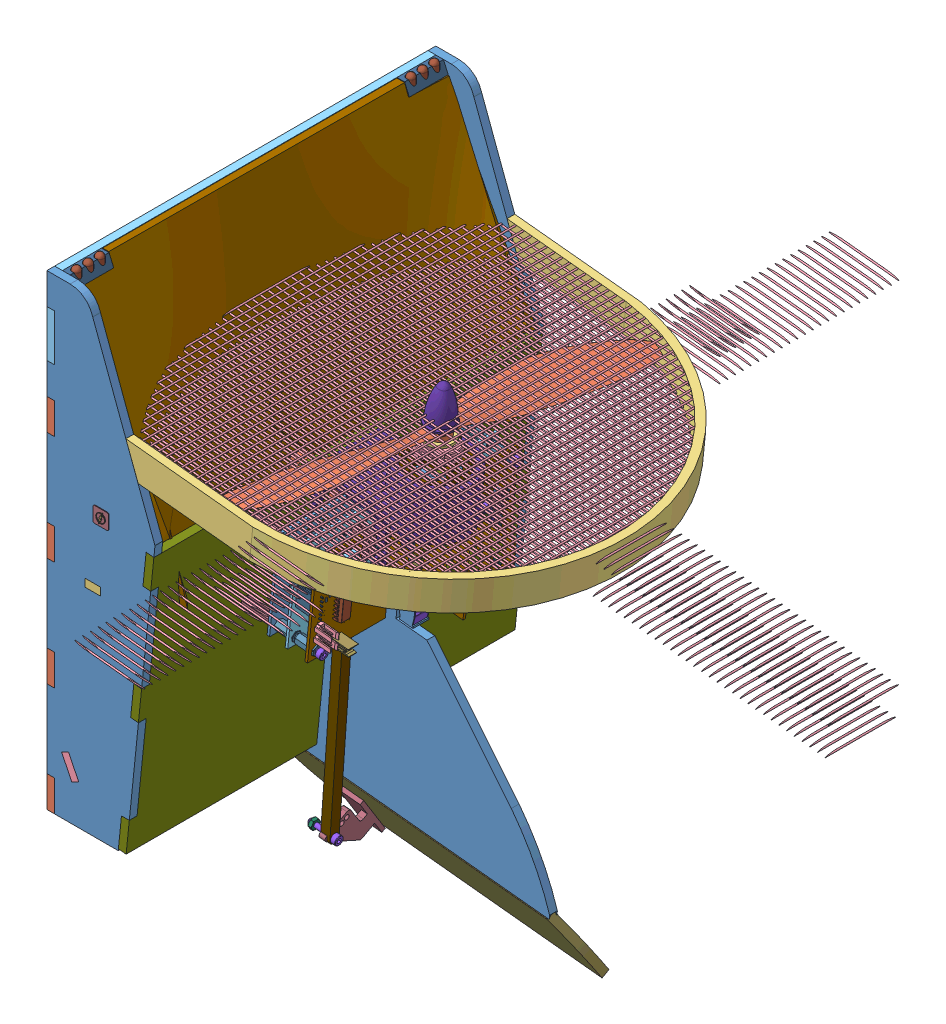
SolidWorks assembly AssTotaleSimu3, configuration Défaut. Lengths in mm.
Overall size (253.25 382.9 251.6).
1779 component instances, 238 part files, 11 mates.
Components (placement in the parent):
- AssStructSimu-1: AssStructSimu [Défaut] at (-125.7658 -1.8483 624.6548) x (1 0 0) z (0 0 -1) size (253.25 324.59 251.6)
  - AssBase-1: AssBase [Défaut] at (36.5482 -71.0398 34.0612) size (86.08 302.3 251.6)
    - AssD-1: AssD [Défaut] at (39.0992 31.0201 8.5) size (69.5 300 22)
      - P1-1: P1 [Défaut] at (-95.5819 194.6656 377.5) size (69.5 300 5)
      - P5-1: P5 [Défaut] at (-100.5819 -35.3344 360.5) x (0 1 0) z (1 0 0) size (230 22 5)
    - AssG-1: AssG [Défaut] at (39.0992 31.0201 -236.5) size (69.5 300 22)
      - P1-1: P1 [Défaut] at (-95.5819 194.6656 377.5) size (69.5 300 5)
      - P5-1: P5 [Défaut] at (-95.5819 -35.3344 399.5) x (0 1 0) z (-1 0 0) size (230 22 5)
    - P7-1: P7 [Défaut] at (-1.4828 89.6857 370.5) x (0 0 -1) z (0 -1 0) size (250 54.5 5)
    - P4-1: P4 [Défaut] at (-63.2363 165.9323 386) x (0 0 -1) z (0.898794 -0.438371 0) size (250 60.5 66.27)
    - P3-1: P3 [Défaut] at (-56.4828 -74.3143 146) x (0 0 1) z (-1 0 0) size (250 70 5)
    - P4b-1: P4b [Défaut] at (-58.7423 163.7404 190) x (0 0 1) z (0.438371 0.898794 0) size (152 56 2)
    - battery-1: battery [Défaut] at (-39.0156 204.1861 197.5) x (0 0 1) z (0.898794 -0.438371 0) size (137 43 30)
    - socket head cap screw 4762_din-1: socket head cap screw 4762_din [EN ISO 4762 M3 x 10 - 10N] at (-27.7008 145.2627 193) x (0.438371 0.898794 0) z (0 0 -1) size (13 5.5 5.5)
    - socket head cap screw 4762_din-2: socket head cap screw 4762_din [EN ISO 4762 M3 x 10 - 10N] at (-27.7008 145.2627 339) x (0.438371 0.898794 0) z (-0.791285 0.385936 -0.474259) size (13 5.5 5.5)
    - socket head cap screw 4762_din-3: socket head cap screw 4762_din [EN ISO 4762 M3 x 10 - 10N] at (-42.0815 152.2766 339) x (0.438371 0.898794 0) z (-0.001489 0.000726 -0.999999) size (13 5.5 5.5)
    - socket head cap screw 4762_din-4: socket head cap screw 4762_din [EN ISO 4762 M3 x 10 - 10N] at (-42.0815 152.2766 193) x (0.438371 0.898794 0) z (-0.031331 0.015281 -0.999392) size (13 5.5 5.5)
    - P11-1: P11 [Défaut] at (-57.5734 -73.9703 146.7843) x (0.005072 0 0.999987) z (0.006197 0.999981 -0.000031) size (240 65 164)
    - AssPhare-1: AssPhare [Défaut] at (-52.8518 -67.6977 411) x (0 1 0) z (0 0 -1) size (40.8 8 27.06)
      - piece_led-1: piece_led [Défaut] at (-6.6166 -3.631 25) size (7 8 25)
      - LED 5mm-1: LED 5mm [Valor predeterminado] at (-0.1166 0.369 30) x (0 0 1) z (-1 0 0) size (10.06 6 40.8)
      - LED 5mm-2: LED 5mm [Valor predeterminado] at (-0.1166 0.369 37.5) x (0 0 1) z (-1 0 0) size (10.06 6 40.8)
      - LED 5mm-3: LED 5mm [Valor predeterminado] at (-0.1166 0.369 45) x (0 0 1) z (-1 0 0) size (10.06 6 40.8)
    - AssPhare-2: AssPhare [Défaut] at (-52.8518 -67.6977 196) x (0 1 0) z (0 0 -1) size (40.8 8 27.06)
      - piece_led-1: piece_led [Défaut] at (-6.6166 -3.631 25) size (7 8 25)
      - LED 5mm-1: LED 5mm [Valor predeterminado] at (-0.1166 0.369 30) x (0 0 1) z (-1 0 0) size (10.06 6 40.8)
      - LED 5mm-2: LED 5mm [Valor predeterminado] at (-0.1166 0.369 37.5) x (0 0 1) z (-1 0 0) size (10.06 6 40.8)
      - LED 5mm-3: LED 5mm [Valor predeterminado] at (-0.1166 0.369 45) x (0 0 1) z (-1 0 0) size (10.06 6 40.8)
    - AssLogo-1: AssLogo [Défaut] at (-27.8835 45.1673 148.1054) x (-1 0 0) z (0 0 -1) size (10 10 0.8)
      - logo1-1: logo1 [Défaut] at (-6.5271 -4.4734 6.5054) size (5.8 7.71 0.4)
      - logo2-1: logo2 [Défaut] at (-6.4007 -4.4815 7.1054) size (10 10 0.4)
    - AssLogo-2: AssLogo [Défaut] at (-25.082 45.1673 383.8946) size (10 10 0.8)
      - logo1-1: logo1 [Défaut] at (-6.5271 -4.4734 6.5054) size (5.8 7.71 0.4)
      - logo2-1: logo2 [Défaut] at (-6.4007 -4.4815 7.1054) size (10 10 0.4)
    - support2-1: support2 [Défaut] at (-61.5648 191.7124 276) x (-0.017452 -0.999848 0) z (0.999848 -0.017452 0) size (75 20 10)
    - socket head cap screw 4762_din-5: socket head cap screw 4762_din [EN ISO 4762 M3 x 5 - 5N] at (-61.652 186.7132 269.3333) x (0.999848 -0.017452 0) z (-0.002158 -0.123615 0.992328) size (8 5.5 5.5)
    - socket head cap screw 4762_din-6: socket head cap screw 4762_din [EN ISO 4762 M3 x 5 - 5N] at (-61.652 186.7132 262.6667) x (0.999848 -0.017452 0) z (0 0 1) size (8 5.5 5.5)
    - socket head cap screw 4762_din-7: socket head cap screw 4762_din [EN ISO 4762 M3 x 25 - 18N] at (-55.2963 121.0922 253) x (0 0 1) z (-1 0 0) size (28 5.5 5.5)
    - hex nut style 1 gradeab_din-1: hex nut style 1 gradeab_din [Hexagon Nut ISO 4032 - M3 - W - N] at (-55.2963 121.0922 276) x (-0.923728 -0.383049 0) z (0 0 -1) size (5.5 6.35 2.4)
  - AssToitMot-1: AssToitMot [Défaut] at (-168.5238 43.6961 238.494) x (0 0 -1) z (0.9948 0.101852 0) size (250 207.5 205)
    - AssToit-1: AssToit [Défaut] at (-23.0702 -16.5789 -3.7148) size (250 207.5 205)
      - P8-1: P8 [Défaut] at (-38.4971 122.5921 203.5) size (250 175 5)
      - P12-1: P12 [Défaut] at (-60.4971 -63.4079 265.5) x (1 0 0) z (0 -1 0) size (44.28 76.64 55)
      - P13-1: P13 [Défaut] at (-35.9971 -52.8579 208.5) x (0 0 1) z (-1 0 0) size (64 15.55 5)
      - P10_2-1: P10_2 [Défaut] at (-35.9971 111.5921 171) x (0 0 1) z (-1 0 0) size (188.5 117.6 5)
    - Parallax-Servo_DUMMY-1: Parallax-Servo_DUMMY [Défaut] at (-61.6002 -51.5207 216.6662) x (1 0 0) z (0 1 0) size (20.07 42.67 55.64)
    - socket head cap screw 4762_din-1: socket head cap screw 4762_din [EN ISO 4762 M2.5 x 5 - 5N] at (-51.9272 -76.4868 259.2852) x (0 -1 0) z (-0.546944 0 0.837169) size (7.5 4.5 4.5)
    - socket head cap screw 4762_din-2: socket head cap screw 4762_din [EN ISO 4762 M2.5 x 5 - 5N] at (-61.5672 -76.4868 268.9252) x (0 -1 0) z (-0.546944 0 0.837169) size (7.5 4.5 4.5)
    - socket head cap screw 4762_din-3: socket head cap screw 4762_din [EN ISO 4762 M2.5 x 5 - 5N] at (-71.2072 -76.4868 259.2852) x (0 -1 0) z (-0.546944 0 0.837169) size (7.5 4.5 4.5)
    - socket head cap screw 4762_din-4: socket head cap screw 4762_din [EN ISO 4762 M2.5 x 5 - 5N] at (-61.5672 -76.4868 249.6452) x (0 -1 0) z (-0.546944 0 0.837169) size (7.5 4.5 4.5)
    - AssPhare-1: AssPhare [Défaut] at (8.4328 83.3966 196.1542) x (0 -1 0) z (1 0 0) size (40.8 8 27.06)
      - piece_led-1: piece_led [Défaut] at (-6.6166 -3.631 25) size (7 8 25)
      - LED 5mm-1: LED 5mm [Valor predeterminado] at (-0.1166 0.369 30) x (0 0 1) z (-1 0 0) size (10.06 6 40.8)
      - LED 5mm-2: LED 5mm [Valor predeterminado] at (-0.1166 0.369 37.5) x (0 0 1) z (-1 0 0) size (10.06 6 40.8)
      - LED 5mm-3: LED 5mm [Valor predeterminado] at (-0.1166 0.369 45) x (0 0 1) z (-1 0 0) size (10.06 6 40.8)
    - AssPhare-2: AssPhare [Défaut] at (-206.5672 83.3966 196.1542) x (0 -1 0) z (1 0 0) size (40.8 8 27.06)
      - piece_led-1: piece_led [Défaut] at (-6.6166 -3.631 25) size (7 8 25)
      - LED 5mm-1: LED 5mm [Valor predeterminado] at (-0.1166 0.369 30) x (0 0 1) z (-1 0 0) size (10.06 6 40.8)
      - LED 5mm-2: LED 5mm [Valor predeterminado] at (-0.1166 0.369 37.5) x (0 0 1) z (-1 0 0) size (10.06 6 40.8)
      - LED 5mm-3: LED 5mm [Valor predeterminado] at (-0.1166 0.369 45) x (0 0 1) z (-1 0 0) size (10.06 6 40.8)
    - socket head cap screw 4762_din-5: socket head cap screw 4762_din [EN ISO 4762 M3 x 10 - 10N] at (-67.0672 -22.9368 210.2852) x (0 0 -1) z (1 0 0) size (13 5.5 5.5)
    - socket head cap screw 4762_din-6: socket head cap screw 4762_din [EN ISO 4762 M3 x 10 - 10N] at (-56.0672 -72.9868 210.2852) x (0 0 -1) z (1 0 0) size (13 5.5 5.5)
    - socket head cap screw 4762_din-7: socket head cap screw 4762_din [EN ISO 4762 M3 x 10 - 10N] at (-67.0672 -72.9868 210.2852) x (0 0 -1) z (1 0 0) size (13 5.5 5.5)
    - socket head cap screw 4762_din-8: socket head cap screw 4762_din [EN ISO 4762 M3 x 10 - 10N] at (-56.0672 -22.9368 210.2852) x (0 0 -1) z (1 0 0) size (13 5.5 5.5)
    - hex nut style 1 gradeab_din-1: hex nut style 1 gradeab_din [Hexagon Nut ISO 4032 - M3 - W - N] at (-67.0672 -72.9868 197.3852) x (-0.923728 -0.383049 0) z (0 0 -1) size (5.5 6.35 2.4)
    - hex nut style 1 gradeab_din-2: hex nut style 1 gradeab_din [Hexagon Nut ISO 4032 - M3 - W - N] at (-56.0672 -72.9868 199.7852) size (5.5 6.35 2.4)
    - hex nut style 1 gradeab_din-3: hex nut style 1 gradeab_din [Hexagon Nut ISO 4032 - M3 - W - N] at (-67.0672 -22.9368 199.7852) size (5.5 6.35 2.4)
    - hex nut style 1 gradeab_din-4: hex nut style 1 gradeab_din [Hexagon Nut ISO 4032 - M3 - W - N] at (-56.0672 -22.9368 199.7852) size (5.5 6.35 2.4)
  - AssProtec-1: AssProtec [Défaut] at (86.6746 190.4649 284.6351) x (0 0 -1) z (0.101852 -0.9948 0) size (250 237.46 20)
    - protec3c-1: protec3c [Défaut] at (-140.4261 -87.7568 240) size (250 197 20)
    - AssGrillage-1: AssGrillage [Défaut] at (-370.4609 -132.5428 258.3161) x (0 0 -1) z (1 0 0) size (2.02 237.05 250)
      - barreau-1: barreau [Défaut] at (-1.1839 0.254 200) size (1 1 400)
      - barreau-3: barreau [Défaut] at (-1.1839 5.254 200) size (1 1 400)
      - barreau-4: barreau [Défaut] at (-1.1839 10.254 200) size (1 1 400)
      - barreau-5: barreau [Défaut] at (-1.1839 15.254 200) size (1 1 400)
      - barreau-6: barreau [Défaut] at (-1.1839 20.254 200) size (1 1 400)
      - barreau-7: barreau [Défaut] at (-1.1839 25.254 200) size (1 1 400)
      - barreau-8: barreau [Défaut] at (-1.1839 30.254 200) size (1 1 400)
      - barreau-9: barreau [Défaut] at (-1.1839 35.254 200) size (1 1 400)
      - barreau-10: barreau [Défaut] at (-1.1839 40.254 200) size (1 1 400)
      - barreau-11: barreau [Défaut] at (-1.1839 45.254 200) size (1 1 400)
      - barreau-12: barreau [Défaut] at (-1.1839 50.254 200) size (1 1 400)
      - barreau-13: barreau [Défaut] at (-1.1839 55.254 200) size (1 1 400)
      - barreau-14: barreau [Défaut] at (-1.1839 60.254 200) size (1 1 400)
      - barreau-15: barreau [Défaut] at (-1.1839 65.254 200) size (1 1 400)
      - barreau-16: barreau [Défaut] at (-1.1839 70.254 200) size (1 1 400)
      - barreau-17: barreau [Défaut] at (-1.1839 75.254 200) size (1 1 400)
      - barreau-18: barreau [Défaut] at (-1.1839 80.254 200) size (1 1 400)
      - barreau-19: barreau [Défaut] at (-1.1839 85.254 200) size (1 1 400)
      - barreau-20: barreau [Défaut] at (-1.1839 90.254 200) size (1 1 400)
      - barreau-21: barreau [Défaut] at (-1.1839 95.254 200) size (1 1 400)
      - barreau-22: barreau [Défaut] at (-1.1839 100.254 200) size (1 1 400)
      - barreau-23: barreau [Défaut] at (-1.1839 105.254 200) size (1 1 400)
      - barreau-24: barreau [Défaut] at (-1.1839 110.254 200) size (1 1 400)
      - barreau-25: barreau [Défaut] at (-1.1839 115.254 200) size (1 1 400)
      - barreau-26: barreau [Défaut] at (-1.1839 120.254 200) size (1 1 400)
      - barreau-27: barreau [Défaut] at (-1.1839 125.254 200) size (1 1 400)
      - barreau-28: barreau [Défaut] at (-1.1839 130.254 200) size (1 1 400)
      - barreau-29: barreau [Défaut] at (-1.1839 135.254 200) size (1 1 400)
      - barreau-30: barreau [Défaut] at (-1.1839 140.254 200) size (1 1 400)
      - barreau-31: barreau [Défaut] at (-1.1839 145.254 200) size (1 1 400)
      - barreau-32: barreau [Défaut] at (-1.1839 150.254 200) size (1 1 400)
      - barreau-33: barreau [Défaut] at (-1.1839 155.254 200) size (1 1 400)
      - barreau-34: barreau [Défaut] at (-1.1839 160.254 200) size (1 1 400)
      - barreau-35: barreau [Défaut] at (-1.1839 165.254 200) size (1 1 400)
      - barreau-36: barreau [Défaut] at (-1.1839 170.254 200) size (1 1 400)
      - barreau-37: barreau [Défaut] at (-1.1839 175.254 200) size (1 1 400)
      - barreau-38: barreau [Défaut] at (-1.1839 180.254 200) size (1 1 400)
      - barreau-39: barreau [Défaut] at (-1.1839 185.254 200) size (1 1 400)
      - barreau-40: barreau [Défaut] at (-1.1839 190.254 200) size (1 1 400)
      - barreau-41: barreau [Défaut] at (-1.1839 195.254 200) size (1 1 400)
      - barreau-42: barreau [Défaut] at (-0.1839 -1.5314 598.7823) x (0.998922 0 0.04641) z (0 1 0) size (1 1 400)
      - barreau-43: barreau [Défaut] at (-1.1839 200.254 200) size (1 1 400)
      - barreau-44: barreau [Défaut] at (-1.1839 205.254 200) size (1 1 400)
      - barreau-45: barreau [Défaut] at (-1.1839 210.254 200) size (1 1 400)
      - barreau-46: barreau [Défaut] at (-1.1839 215.254 200) size (1 1 400)
      - barreau-47: barreau [Défaut] at (-1.1839 220.254 200) size (1 1 400)
      - barreau-48: barreau [Défaut] at (-1.1839 225.254 200) size (1 1 400)
      - barreau-49: barreau [Défaut] at (-1.1839 230.254 200) size (1 1 400)
      - barreau-50: barreau [Défaut] at (-1.1839 235.254 200) size (1 1 400)
      - barreau-51: barreau [Défaut] at (-1.1839 240.254 200) size (1 1 400)
      - barreau-52: barreau [Défaut] at (-1.1839 245.254 200) size (1 1 400)
      - barreau-53: barreau [Défaut] at (-1.1839 250.254 200) size (1 1 400)
      - barreau-54: barreau [Défaut] at (-1.1839 255.254 200) size (1 1 400)
      - barreau-55: barreau [Défaut] at (-1.1839 260.254 200) size (1 1 400)
      - barreau-56: barreau [Défaut] at (-1.1839 265.254 200) size (1 1 400)
      - barreau-57: barreau [Défaut] at (-1.1839 270.254 200) size (1 1 400)
      - barreau-58: barreau [Défaut] at (-1.1839 275.254 200) size (1 1 400)
      - barreau-59: barreau [Défaut] at (-1.1839 280.254 200) size (1 1 400)
      - barreau-60: barreau [Défaut] at (-1.1839 285.254 200) size (1 1 400)
      - barreau-61: barreau [Défaut] at (-1.1839 290.254 200) size (1 1 400)
      - barreau-62: barreau [Défaut] at (-1.1839 295.254 200) size (1 1 400)
      - barreau-63: barreau [Défaut] at (-1.1839 300.254 200) size (1 1 400)
      - barreau-64: barreau [Défaut] at (-1.1839 305.254 200) size (1 1 400)
      - barreau-65: barreau [Défaut] at (-1.1839 310.254 200) size (1 1 400)
      - barreau-66: barreau [Défaut] at (-1.1839 315.254 200) size (1 1 400)
      - barreau-67: barreau [Défaut] at (-1.1839 320.254 200) size (1 1 400)
      - barreau-68: barreau [Défaut] at (-1.1839 325.254 200) size (1 1 400)
      - barreau-69: barreau [Défaut] at (-1.1839 330.254 200) size (1 1 400)
      - barreau-70: barreau [Défaut] at (-1.1839 335.254 200) size (1 1 400)
      - barreau-71: barreau [Défaut] at (-1.1839 340.254 200) size (1 1 400)
      - barreau-72: barreau [Défaut] at (-1.1839 345.254 200) size (1 1 400)
      - barreau-73: barreau [Défaut] at (-1.1839 350.254 200) size (1 1 400)
      - barreau-74: barreau [Défaut] at (-1.1839 355.254 200) size (1 1 400)
      - barreau-75: barreau [Défaut] at (-1.1839 360.254 200) size (1 1 400)
      - barreau-76: barreau [Défaut] at (-1.1839 365.254 200) size (1 1 400)
      - barreau-77: barreau [Défaut] at (-1.1839 370.254 200) size (1 1 400)
      - barreau-78: barreau [Défaut] at (-1.1839 375.254 200) size (1 1 400)
      - barreau-79: barreau [Défaut] at (-1.1839 380.254 200) size (1 1 400)
      - barreau-80: barreau [Défaut] at (-1.1839 385.254 200) size (1 1 400)
      - barreau-81: barreau [Défaut] at (-1.1839 390.254 200) size (1 1 400)
      - barreau-82: barreau [Défaut] at (-1.1839 395.254 200) size (1 1 400)
      - barreau-136: barreau [Défaut] at (-0.1839 -1.5314 593.7823) x (0.998922 0 0.04641) z (0 1 0) size (1 1 400)
      - barreau-137: barreau [Défaut] at (-0.1839 -1.5314 588.7823) x (0.998922 0 0.04641) z (0 1 0) size (1 1 400)
      - barreau-138: barreau [Défaut] at (-0.1839 -1.5314 583.7823) x (0.998922 0 0.04641) z (0 1 0) size (1 1 400)
      - barreau-139: barreau [Défaut] at (-0.1839 -1.5314 578.7823) x (0.998922 0 0.04641) z (0 1 0) size (1 1 400)
      - barreau-140: barreau [Défaut] at (-0.1839 -1.5314 573.7823) x (0.998922 0 0.04641) z (0 1 0) size (1 1 400)
      - barreau-141: barreau [Défaut] at (-0.1839 -1.5314 568.7823) x (0.998922 0 0.04641) z (0 1 0) size (1 1 400)
      - barreau-142: barreau [Défaut] at (-0.1839 -1.5314 563.7823) x (0.998922 0 0.04641) z (0 1 0) size (1 1 400)
      - barreau-143: barreau [Défaut] at (-0.1839 -1.5314 558.7823) x (0.998922 0 0.04641) z (0 1 0) size (1 1 400)
      - barreau-144: barreau [Défaut] at (-0.1839 -1.5314 553.7823) x (0.998922 0 0.04641) z (0 1 0) size (1 1 400)
      - barreau-145: barreau [Défaut] at (-0.1839 -1.5314 548.7823) x (0.998922 0 0.04641) z (0 1 0) size (1 1 400)
      - barreau-146: barreau [Défaut] at (-0.1839 -1.5314 543.7823) x (0.998922 0 0.04641) z (0 1 0) size (1 1 400)
      - barreau-147: barreau [Défaut] at (-0.1839 -1.5314 538.7823) x (0.998922 0 0.04641) z (0 1 0) size (1 1 400)
      - barreau-148: barreau [Défaut] at (-0.1839 -1.5314 533.7823) x (0.998922 0 0.04641) z (0 1 0) size (1 1 400)
      - barreau-149: barreau [Défaut] at (-0.1839 -1.5314 528.7823) x (0.998922 0 0.04641) z (0 1 0) size (1 1 400)
      - barreau-150: barreau [Défaut] at (-0.1839 -1.5314 523.7823) x (0.998922 0 0.04641) z (0 1 0) size (1 1 400)
      - barreau-151: barreau [Défaut] at (-0.1839 -1.5314 518.7823) x (0.998922 0 0.04641) z (0 1 0) size (1 1 400)
      - barreau-152: barreau [Défaut] at (-0.1839 -1.5314 513.7823) x (0.998922 0 0.04641) z (0 1 0) size (1 1 400)
      - barreau-153: barreau [Défaut] at (-0.1839 -1.5314 508.7823) x (0.998922 0 0.04641) z (0 1 0) size (1 1 400)
      - barreau-154: barreau [Défaut] at (-0.1839 -1.5314 503.7823) x (0.998922 0 0.04641) z (0 1 0) size (1 1 400)
      - barreau-155: barreau [Défaut] at (-0.1839 -1.5314 498.7823) x (0.998922 0 0.04641) z (0 1 0) size (1 1 400)
      - barreau-156: barreau [Défaut] at (-0.1839 -1.5314 493.7823) x (0.998922 0 0.04641) z (0 1 0) size (1 1 400)
      - barreau-157: barreau [Défaut] at (-0.1839 -1.5314 488.7823) x (0.998922 0 0.04641) z (0 1 0) size (1 1 400)
      - barreau-158: barreau [Défaut] at (-0.1839 -1.5314 483.7823) x (0.998922 0 0.04641) z (0 1 0) size (1 1 400)
      - barreau-159: barreau [Défaut] at (-0.1839 -1.5314 478.7823) x (0.998922 0 0.04641) z (0 1 0) size (1 1 400)
      - barreau-160: barreau [Défaut] at (-0.1839 -1.5314 473.7823) x (0.998922 0 0.04641) z (0 1 0) size (1 1 400)
      - barreau-161: barreau [Défaut] at (-0.1839 -1.5314 468.7823) x (0.998922 0 0.04641) z (0 1 0) size (1 1 400)
      - barreau-162: barreau [Défaut] at (-0.1839 -1.5314 463.7823) x (0.998922 0 0.04641) z (0 1 0) size (1 1 400)
      - barreau-163: barreau [Défaut] at (-0.1839 -1.5314 458.7823) x (0.998922 0 0.04641) z (0 1 0) size (1 1 400)
      - barreau-164: barreau [Défaut] at (-0.1839 -1.5314 453.7823) x (0.998922 0 0.04641) z (0 1 0) size (1 1 400)
      - barreau-165: barreau [Défaut] at (-0.1839 -1.5314 448.7823) x (0.998922 0 0.04641) z (0 1 0) size (1 1 400)
      - barreau-166: barreau [Défaut] at (-0.1839 -1.5314 443.7823) x (0.998922 0 0.04641) z (0 1 0) size (1 1 400)
      - barreau-167: barreau [Défaut] at (-0.1839 -1.5314 438.7823) x (0.998922 0 0.04641) z (0 1 0) size (1 1 400)
      - barreau-168: barreau [Défaut] at (-0.1839 -1.5314 433.7823) x (0.998922 0 0.04641) z (0 1 0) size (1 1 400)
      - barreau-169: barreau [Défaut] at (-0.1839 -1.5314 428.7823) x (0.998922 0 0.04641) z (0 1 0) size (1 1 400)
      - barreau-170: barreau [Défaut] at (-0.1839 -1.5314 423.7823) x (0.998922 0 0.04641) z (0 1 0) size (1 1 400)
      - barreau-171: barreau [Défaut] at (-0.1839 -1.5314 418.7823) x (0.998922 0 0.04641) z (0 1 0) size (1 1 400)
      - barreau-172: barreau [Défaut] at (-0.1839 -1.5314 413.7823) x (0.998922 0 0.04641) z (0 1 0) size (1 1 400)
      - barreau-173: barreau [Défaut] at (-0.1839 -1.5314 408.7823) x (0.998922 0 0.04641) z (0 1 0) size (1 1 400)
      - barreau-174: barreau [Défaut] at (-0.1839 -1.5314 403.7823) x (0.998922 0 0.04641) z (0 1 0) size (1 1 400)
      - barreau-175: barreau [Défaut] at (-0.1839 -1.5314 398.7823) x (0.998922 0 0.04641) z (0 1 0) size (1 1 400)
      - barreau-176: barreau [Défaut] at (-0.1839 -1.5314 393.7823) x (0.998922 0 0.04641) z (0 1 0) size (1 1 400)
      - barreau-177: barreau [Défaut] at (-0.1839 -1.5314 388.7823) x (0.998922 0 0.04641) z (0 1 0) size (1 1 400)
      - barreau-178: barreau [Défaut] at (-0.1839 -1.5314 383.7823) x (0.998922 0 0.04641) z (0 1 0) size (1 1 400)
      - barreau-179: barreau [Défaut] at (-0.1839 -1.5314 378.7823) x (0.998922 0 0.04641) z (0 1 0) size (1 1 400)
      - barreau-180: barreau [Défaut] at (-0.1839 -1.5314 373.7823) x (0.998922 0 0.04641) z (0 1 0) size (1 1 400)
      - barreau-181: barreau [Défaut] at (-0.1839 -1.5314 368.7823) x (0.998922 0 0.04641) z (0 1 0) size (1 1 400)
      - barreau-182: barreau [Défaut] at (-0.1839 -1.5314 363.7823) x (0.998922 0 0.04641) z (0 1 0) size (1 1 400)
      - barreau-183: barreau [Défaut] at (-0.1839 -1.5314 358.7823) x (0.998922 0 0.04641) z (0 1 0) size (1 1 400)
      - barreau-184: barreau [Défaut] at (-0.1839 -1.5314 353.7823) x (0.998922 0 0.04641) z (0 1 0) size (1 1 400)
      - barreau-185: barreau [Défaut] at (-0.1839 -1.5314 348.7823) x (0.998922 0 0.04641) z (0 1 0) size (1 1 400)
      - barreau-186: barreau [Défaut] at (-0.1839 -1.5314 343.7823) x (0.998922 0 0.04641) z (0 1 0) size (1 1 400)
      - barreau-187: barreau [Défaut] at (-0.1839 -1.5314 338.7823) x (0.998922 0 0.04641) z (0 1 0) size (1 1 400)
      - barreau-188: barreau [Défaut] at (-0.1839 -1.5314 333.7823) x (0.998922 0 0.04641) z (0 1 0) size (1 1 400)
      - barreau-189: barreau [Défaut] at (-0.1839 -1.5314 328.7823) x (0.998922 0 0.04641) z (0 1 0) size (1 1 400)
      - barreau-190: barreau [Défaut] at (-0.1839 -1.5314 323.7823) x (0.998922 0 0.04641) z (0 1 0) size (1 1 400)
      - barreau-191: barreau [Défaut] at (-0.1839 -1.5314 318.7823) x (0.998922 0 0.04641) z (0 1 0) size (1 1 400)
      - barreau-192: barreau [Défaut] at (-0.1839 -1.5314 313.7823) x (0.998922 0 0.04641) z (0 1 0) size (1 1 400)
      - barreau-193: barreau [Défaut] at (-0.1839 -1.5314 308.7823) x (0.998922 0 0.04641) z (0 1 0) size (1 1 400)
      - barreau-194: barreau [Défaut] at (-0.1839 -1.5314 303.7823) x (0.998922 0 0.04641) z (0 1 0) size (1 1 400)
      - barreau-195: barreau [Défaut] at (-0.1839 -1.5314 298.7823) x (0.998922 0 0.04641) z (0 1 0) size (1 1 400)
      - barreau-196: barreau [Défaut] at (-0.1839 -1.5314 293.7823) x (0.998922 0 0.04641) z (0 1 0) size (1 1 400)
      - barreau-197: barreau [Défaut] at (-0.1839 -1.5314 288.7823) x (0.998922 0 0.04641) z (0 1 0) size (1 1 400)
      - barreau-198: barreau [Défaut] at (-0.1839 -1.5314 283.7823) x (0.998922 0 0.04641) z (0 1 0) size (1 1 400)
      - barreau-199: barreau [Défaut] at (-0.1839 -1.5314 278.7823) x (0.998922 0 0.04641) z (0 1 0) size (1 1 400)
      - barreau-200: barreau [Défaut] at (-0.1839 -1.5314 273.7823) x (0.998922 0 0.04641) z (0 1 0) size (1 1 400)
      - barreau-201: barreau [Défaut] at (-0.1839 -1.5314 268.7823) x (0.998922 0 0.04641) z (0 1 0) size (1 1 400)
      - barreau-202: barreau [Défaut] at (-0.1839 -1.5314 263.7823) x (0.998922 0 0.04641) z (0 1 0) size (1 1 400)
      - barreau-203: barreau [Défaut] at (-0.1839 -1.5314 258.7823) x (0.998922 0 0.04641) z (0 1 0) size (1 1 400)
      - barreau-204: barreau [Défaut] at (-0.1839 -1.5314 253.7823) x (0.998922 0 0.04641) z (0 1 0) size (1 1 400)
      - barreau-205: barreau [Défaut] at (-0.1839 -1.5314 248.7823) x (0.998922 0 0.04641) z (0 1 0) size (1 1 400)
      - barreau-206: barreau [Défaut] at (-0.1839 -1.5314 243.7823) x (0.998922 0 0.04641) z (0 1 0) size (1 1 400)
      - barreau-207: barreau [Défaut] at (-0.1839 -1.5314 238.7823) x (0.998922 0 0.04641) z (0 1 0) size (1 1 400)
      - barreau-208: barreau [Défaut] at (-0.1839 -1.5314 233.7823) x (0.998922 0 0.04641) z (0 1 0) size (1 1 400)
      - barreau-209: barreau [Défaut] at (-0.1839 -1.5314 228.7823) x (0.998922 0 0.04641) z (0 1 0) size (1 1 400)
      - barreau-210: barreau [Défaut] at (-0.1839 -1.5314 223.7823) x (0.998922 0 0.04641) z (0 1 0) size (1 1 400)
      - barreau-211: barreau [Défaut] at (-0.1839 -1.5314 218.7823) x (0.998922 0 0.04641) z (0 1 0) size (1 1 400)
      - barreau-212: barreau [Défaut] at (-0.1839 -1.5314 213.7823) x (0.998922 0 0.04641) z (0 1 0) size (1 1 400)
      - barreau-213: barreau [Défaut] at (-0.1839 -1.5314 208.7823) x (0.998922 0 0.04641) z (0 1 0) size (1 1 400)
      - barreau-214: barreau [Défaut] at (-0.1839 -1.5314 203.7823) x (0.998922 0 0.04641) z (0 1 0) size (1 1 400)
    - AssGrillage-2: AssGrillage [Défaut] at (339.6086 -132.5428 241.6839) x (0 0 1) z (-1 0 0) size (2.02 237.05 250)
      - barreau-1: barreau [Défaut] at (-1.1839 0.254 200) size (1 1 400)
      - barreau-3: barreau [Défaut] at (-1.1839 5.254 200) size (1 1 400)
      - barreau-4: barreau [Défaut] at (-1.1839 10.254 200) size (1 1 400)
      - barreau-5: barreau [Défaut] at (-1.1839 15.254 200) size (1 1 400)
      - barreau-6: barreau [Défaut] at (-1.1839 20.254 200) size (1 1 400)
      - barreau-7: barreau [Défaut] at (-1.1839 25.254 200) size (1 1 400)
      - barreau-8: barreau [Défaut] at (-1.1839 30.254 200) size (1 1 400)
      - barreau-9: barreau [Défaut] at (-1.1839 35.254 200) size (1 1 400)
      - barreau-10: barreau [Défaut] at (-1.1839 40.254 200) size (1 1 400)
      - barreau-11: barreau [Défaut] at (-1.1839 45.254 200) size (1 1 400)
      - barreau-12: barreau [Défaut] at (-1.1839 50.254 200) size (1 1 400)
      - barreau-13: barreau [Défaut] at (-1.1839 55.254 200) size (1 1 400)
      - barreau-14: barreau [Défaut] at (-1.1839 60.254 200) size (1 1 400)
      - barreau-15: barreau [Défaut] at (-1.1839 65.254 200) size (1 1 400)
      - barreau-16: barreau [Défaut] at (-1.1839 70.254 200) size (1 1 400)
      - barreau-17: barreau [Défaut] at (-1.1839 75.254 200) size (1 1 400)
      - barreau-18: barreau [Défaut] at (-1.1839 80.254 200) size (1 1 400)
      - barreau-19: barreau [Défaut] at (-1.1839 85.254 200) size (1 1 400)
      - barreau-20: barreau [Défaut] at (-1.1839 90.254 200) size (1 1 400)
      - barreau-21: barreau [Défaut] at (-1.1839 95.254 200) size (1 1 400)
      - barreau-22: barreau [Défaut] at (-1.1839 100.254 200) size (1 1 400)
      - barreau-23: barreau [Défaut] at (-1.1839 105.254 200) size (1 1 400)
      - barreau-24: barreau [Défaut] at (-1.1839 110.254 200) size (1 1 400)
      - barreau-25: barreau [Défaut] at (-1.1839 115.254 200) size (1 1 400)
      - barreau-26: barreau [Défaut] at (-1.1839 120.254 200) size (1 1 400)
      - barreau-27: barreau [Défaut] at (-1.1839 125.254 200) size (1 1 400)
      - barreau-28: barreau [Défaut] at (-1.1839 130.254 200) size (1 1 400)
      - barreau-29: barreau [Défaut] at (-1.1839 135.254 200) size (1 1 400)
      - barreau-30: barreau [Défaut] at (-1.1839 140.254 200) size (1 1 400)
      - barreau-31: barreau [Défaut] at (-1.1839 145.254 200) size (1 1 400)
      - barreau-32: barreau [Défaut] at (-1.1839 150.254 200) size (1 1 400)
      - barreau-33: barreau [Défaut] at (-1.1839 155.254 200) size (1 1 400)
      - barreau-34: barreau [Défaut] at (-1.1839 160.254 200) size (1 1 400)
      - barreau-35: barreau [Défaut] at (-1.1839 165.254 200) size (1 1 400)
      - barreau-36: barreau [Défaut] at (-1.1839 170.254 200) size (1 1 400)
      - barreau-37: barreau [Défaut] at (-1.1839 175.254 200) size (1 1 400)
      - barreau-38: barreau [Défaut] at (-1.1839 180.254 200) size (1 1 400)
      - barreau-39: barreau [Défaut] at (-1.1839 185.254 200) size (1 1 400)
      - barreau-40: barreau [Défaut] at (-1.1839 190.254 200) size (1 1 400)
      - barreau-41: barreau [Défaut] at (-1.1839 195.254 200) size (1 1 400)
      - barreau-42: barreau [Défaut] at (-0.1839 -1.5314 598.7823) x (0.998922 0 0.04641) z (0 1 0) size (1 1 400)
      - barreau-43: barreau [Défaut] at (-1.1839 200.254 200) size (1 1 400)
      - barreau-44: barreau [Défaut] at (-1.1839 205.254 200) size (1 1 400)
      - barreau-45: barreau [Défaut] at (-1.1839 210.254 200) size (1 1 400)
      - barreau-46: barreau [Défaut] at (-1.1839 215.254 200) size (1 1 400)
      - barreau-47: barreau [Défaut] at (-1.1839 220.254 200) size (1 1 400)
      - barreau-48: barreau [Défaut] at (-1.1839 225.254 200) size (1 1 400)
      - barreau-49: barreau [Défaut] at (-1.1839 230.254 200) size (1 1 400)
      - barreau-50: barreau [Défaut] at (-1.1839 235.254 200) size (1 1 400)
      - barreau-51: barreau [Défaut] at (-1.1839 240.254 200) size (1 1 400)
      - barreau-52: barreau [Défaut] at (-1.1839 245.254 200) size (1 1 400)
      - barreau-53: barreau [Défaut] at (-1.1839 250.254 200) size (1 1 400)
      - barreau-54: barreau [Défaut] at (-1.1839 255.254 200) size (1 1 400)
      - barreau-55: barreau [Défaut] at (-1.1839 260.254 200) size (1 1 400)
      - barreau-56: barreau [Défaut] at (-1.1839 265.254 200) size (1 1 400)
      - barreau-57: barreau [Défaut] at (-1.1839 270.254 200) size (1 1 400)
      - barreau-58: barreau [Défaut] at (-1.1839 275.254 200) size (1 1 400)
      - barreau-59: barreau [Défaut] at (-1.1839 280.254 200) size (1 1 400)
      - barreau-60: barreau [Défaut] at (-1.1839 285.254 200) size (1 1 400)
      - barreau-61: barreau [Défaut] at (-1.1839 290.254 200) size (1 1 400)
      - barreau-62: barreau [Défaut] at (-1.1839 295.254 200) size (1 1 400)
      - barreau-63: barreau [Défaut] at (-1.1839 300.254 200) size (1 1 400)
      - barreau-64: barreau [Défaut] at (-1.1839 305.254 200) size (1 1 400)
      - barreau-65: barreau [Défaut] at (-1.1839 310.254 200) size (1 1 400)
      - barreau-66: barreau [Défaut] at (-1.1839 315.254 200) size (1 1 400)
      - barreau-67: barreau [Défaut] at (-1.1839 320.254 200) size (1 1 400)
      - barreau-68: barreau [Défaut] at (-1.1839 325.254 200) size (1 1 400)
      - barreau-69: barreau [Défaut] at (-1.1839 330.254 200) size (1 1 400)
      - barreau-70: barreau [Défaut] at (-1.1839 335.254 200) size (1 1 400)
      - barreau-71: barreau [Défaut] at (-1.1839 340.254 200) size (1 1 400)
      - barreau-72: barreau [Défaut] at (-1.1839 345.254 200) size (1 1 400)
      - barreau-73: barreau [Défaut] at (-1.1839 350.254 200) size (1 1 400)
      - barreau-74: barreau [Défaut] at (-1.1839 355.254 200) size (1 1 400)
      - barreau-75: barreau [Défaut] at (-1.1839 360.254 200) size (1 1 400)
      - barreau-76: barreau [Défaut] at (-1.1839 365.254 200) size (1 1 400)
      - barreau-77: barreau [Défaut] at (-1.1839 370.254 200) size (1 1 400)
      - barreau-78: barreau [Défaut] at (-1.1839 375.254 200) size (1 1 400)
      - barreau-79: barreau [Défaut] at (-1.1839 380.254 200) size (1 1 400)
      - barreau-80: barreau [Défaut] at (-1.1839 385.254 200) size (1 1 400)
      - barreau-81: barreau [Défaut] at (-1.1839 390.254 200) size (1 1 400)
      - barreau-82: barreau [Défaut] at (-1.1839 395.254 200) size (1 1 400)
      - barreau-136: barreau [Défaut] at (-0.1839 -1.5314 593.7823) x (0.998922 0 0.04641) z (0 1 0) size (1 1 400)
      - barreau-137: barreau [Défaut] at (-0.1839 -1.5314 588.7823) x (0.998922 0 0.04641) z (0 1 0) size (1 1 400)
      - barreau-138: barreau [Défaut] at (-0.1839 -1.5314 583.7823) x (0.998922 0 0.04641) z (0 1 0) size (1 1 400)
      - barreau-139: barreau [Défaut] at (-0.1839 -1.5314 578.7823) x (0.998922 0 0.04641) z (0 1 0) size (1 1 400)
      - barreau-140: barreau [Défaut] at (-0.1839 -1.5314 573.7823) x (0.998922 0 0.04641) z (0 1 0) size (1 1 400)
      - barreau-141: barreau [Défaut] at (-0.1839 -1.5314 568.7823) x (0.998922 0 0.04641) z (0 1 0) size (1 1 400)
      - barreau-142: barreau [Défaut] at (-0.1839 -1.5314 563.7823) x (0.998922 0 0.04641) z (0 1 0) size (1 1 400)
      - barreau-143: barreau [Défaut] at (-0.1839 -1.5314 558.7823) x (0.998922 0 0.04641) z (0 1 0) size (1 1 400)
      - barreau-144: barreau [Défaut] at (-0.1839 -1.5314 553.7823) x (0.998922 0 0.04641) z (0 1 0) size (1 1 400)
      - barreau-145: barreau [Défaut] at (-0.1839 -1.5314 548.7823) x (0.998922 0 0.04641) z (0 1 0) size (1 1 400)
      - barreau-146: barreau [Défaut] at (-0.1839 -1.5314 543.7823) x (0.998922 0 0.04641) z (0 1 0) size (1 1 400)
      - barreau-147: barreau [Défaut] at (-0.1839 -1.5314 538.7823) x (0.998922 0 0.04641) z (0 1 0) size (1 1 400)
      - barreau-148: barreau [Défaut] at (-0.1839 -1.5314 533.7823) x (0.998922 0 0.04641) z (0 1 0) size (1 1 400)
      - barreau-149: barreau [Défaut] at (-0.1839 -1.5314 528.7823) x (0.998922 0 0.04641) z (0 1 0) size (1 1 400)
      - barreau-150: barreau [Défaut] at (-0.1839 -1.5314 523.7823) x (0.998922 0 0.04641) z (0 1 0) size (1 1 400)
      - barreau-151: barreau [Défaut] at (-0.1839 -1.5314 518.7823) x (0.998922 0 0.04641) z (0 1 0) size (1 1 400)
      - barreau-152: barreau [Défaut] at (-0.1839 -1.5314 513.7823) x (0.998922 0 0.04641) z (0 1 0) size (1 1 400)
      - barreau-153: barreau [Défaut] at (-0.1839 -1.5314 508.7823) x (0.998922 0 0.04641) z (0 1 0) size (1 1 400)
      - barreau-154: barreau [Défaut] at (-0.1839 -1.5314 503.7823) x (0.998922 0 0.04641) z (0 1 0) size (1 1 400)
      - barreau-155: barreau [Défaut] at (-0.1839 -1.5314 498.7823) x (0.998922 0 0.04641) z (0 1 0) size (1 1 400)
      - barreau-156: barreau [Défaut] at (-0.1839 -1.5314 493.7823) x (0.998922 0 0.04641) z (0 1 0) size (1 1 400)
      - barreau-157: barreau [Défaut] at (-0.1839 -1.5314 488.7823) x (0.998922 0 0.04641) z (0 1 0) size (1 1 400)
      - barreau-158: barreau [Défaut] at (-0.1839 -1.5314 483.7823) x (0.998922 0 0.04641) z (0 1 0) size (1 1 400)
      - barreau-159: barreau [Défaut] at (-0.1839 -1.5314 478.7823) x (0.998922 0 0.04641) z (0 1 0) size (1 1 400)
      - barreau-160: barreau [Défaut] at (-0.1839 -1.5314 473.7823) x (0.998922 0 0.04641) z (0 1 0) size (1 1 400)
      - barreau-161: barreau [Défaut] at (-0.1839 -1.5314 468.7823) x (0.998922 0 0.04641) z (0 1 0) size (1 1 400)
      - barreau-162: barreau [Défaut] at (-0.1839 -1.5314 463.7823) x (0.998922 0 0.04641) z (0 1 0) size (1 1 400)
      - barreau-163: barreau [Défaut] at (-0.1839 -1.5314 458.7823) x (0.998922 0 0.04641) z (0 1 0) size (1 1 400)
      - barreau-164: barreau [Défaut] at (-0.1839 -1.5314 453.7823) x (0.998922 0 0.04641) z (0 1 0) size (1 1 400)
      - barreau-165: barreau [Défaut] at (-0.1839 -1.5314 448.7823) x (0.998922 0 0.04641) z (0 1 0) size (1 1 400)
      - barreau-166: barreau [Défaut] at (-0.1839 -1.5314 443.7823) x (0.998922 0 0.04641) z (0 1 0) size (1 1 400)
      - barreau-167: barreau [Défaut] at (-0.1839 -1.5314 438.7823) x (0.998922 0 0.04641) z (0 1 0) size (1 1 400)
      - barreau-168: barreau [Défaut] at (-0.1839 -1.5314 433.7823) x (0.998922 0 0.04641) z (0 1 0) size (1 1 400)
      - barreau-169: barreau [Défaut] at (-0.1839 -1.5314 428.7823) x (0.998922 0 0.04641) z (0 1 0) size (1 1 400)
      - barreau-170: barreau [Défaut] at (-0.1839 -1.5314 423.7823) x (0.998922 0 0.04641) z (0 1 0) size (1 1 400)
      - barreau-171: barreau [Défaut] at (-0.1839 -1.5314 418.7823) x (0.998922 0 0.04641) z (0 1 0) size (1 1 400)
      - barreau-172: barreau [Défaut] at (-0.1839 -1.5314 413.7823) x (0.998922 0 0.04641) z (0 1 0) size (1 1 400)
      - barreau-173: barreau [Défaut] at (-0.1839 -1.5314 408.7823) x (0.998922 0 0.04641) z (0 1 0) size (1 1 400)
      - barreau-174: barreau [Défaut] at (-0.1839 -1.5314 403.7823) x (0.998922 0 0.04641) z (0 1 0) size (1 1 400)
      - barreau-175: barreau [Défaut] at (-0.1839 -1.5314 398.7823) x (0.998922 0 0.04641) z (0 1 0) size (1 1 400)
      - barreau-176: barreau [Défaut] at (-0.1839 -1.5314 393.7823) x (0.998922 0 0.04641) z (0 1 0) size (1 1 400)
      - barreau-177: barreau [Défaut] at (-0.1839 -1.5314 388.7823) x (0.998922 0 0.04641) z (0 1 0) size (1 1 400)
      - barreau-178: barreau [Défaut] at (-0.1839 -1.5314 383.7823) x (0.998922 0 0.04641) z (0 1 0) size (1 1 400)
      - barreau-179: barreau [Défaut] at (-0.1839 -1.5314 378.7823) x (0.998922 0 0.04641) z (0 1 0) size (1 1 400)
      - barreau-180: barreau [Défaut] at (-0.1839 -1.5314 373.7823) x (0.998922 0 0.04641) z (0 1 0) size (1 1 400)
      - barreau-181: barreau [Défaut] at (-0.1839 -1.5314 368.7823) x (0.998922 0 0.04641) z (0 1 0) size (1 1 400)
      - barreau-182: barreau [Défaut] at (-0.1839 -1.5314 363.7823) x (0.998922 0 0.04641) z (0 1 0) size (1 1 400)
      - barreau-183: barreau [Défaut] at (-0.1839 -1.5314 358.7823) x (0.998922 0 0.04641) z (0 1 0) size (1 1 400)
      - barreau-184: barreau [Défaut] at (-0.1839 -1.5314 353.7823) x (0.998922 0 0.04641) z (0 1 0) size (1 1 400)
      - barreau-185: barreau [Défaut] at (-0.1839 -1.5314 348.7823) x (0.998922 0 0.04641) z (0 1 0) size (1 1 400)
      - barreau-186: barreau [Défaut] at (-0.1839 -1.5314 343.7823) x (0.998922 0 0.04641) z (0 1 0) size (1 1 400)
      - barreau-187: barreau [Défaut] at (-0.1839 -1.5314 338.7823) x (0.998922 0 0.04641) z (0 1 0) size (1 1 400)
      - barreau-188: barreau [Défaut] at (-0.1839 -1.5314 333.7823) x (0.998922 0 0.04641) z (0 1 0) size (1 1 400)
      - barreau-189: barreau [Défaut] at (-0.1839 -1.5314 328.7823) x (0.998922 0 0.04641) z (0 1 0) size (1 1 400)
      - barreau-190: barreau [Défaut] at (-0.1839 -1.5314 323.7823) x (0.998922 0 0.04641) z (0 1 0) size (1 1 400)
      - barreau-191: barreau [Défaut] at (-0.1839 -1.5314 318.7823) x (0.998922 0 0.04641) z (0 1 0) size (1 1 400)
      - barreau-192: barreau [Défaut] at (-0.1839 -1.5314 313.7823) x (0.998922 0 0.04641) z (0 1 0) size (1 1 400)
      - barreau-193: barreau [Défaut] at (-0.1839 -1.5314 308.7823) x (0.998922 0 0.04641) z (0 1 0) size (1 1 400)
      - barreau-194: barreau [Défaut] at (-0.1839 -1.5314 303.7823) x (0.998922 0 0.04641) z (0 1 0) size (1 1 400)
      - barreau-195: barreau [Défaut] at (-0.1839 -1.5314 298.7823) x (0.998922 0 0.04641) z (0 1 0) size (1 1 400)
      - barreau-196: barreau [Défaut] at (-0.1839 -1.5314 293.7823) x (0.998922 0 0.04641) z (0 1 0) size (1 1 400)
      - barreau-197: barreau [Défaut] at (-0.1839 -1.5314 288.7823) x (0.998922 0 0.04641) z (0 1 0) size (1 1 400)
      - barreau-198: barreau [Défaut] at (-0.1839 -1.5314 283.7823) x (0.998922 0 0.04641) z (0 1 0) size (1 1 400)
      - barreau-199: barreau [Défaut] at (-0.1839 -1.5314 278.7823) x (0.998922 0 0.04641) z (0 1 0) size (1 1 400)
      - barreau-200: barreau [Défaut] at (-0.1839 -1.5314 273.7823) x (0.998922 0 0.04641) z (0 1 0) size (1 1 400)
      - barreau-201: barreau [Défaut] at (-0.1839 -1.5314 268.7823) x (0.998922 0 0.04641) z (0 1 0) size (1 1 400)
      - barreau-202: barreau [Défaut] at (-0.1839 -1.5314 263.7823) x (0.998922 0 0.04641) z (0 1 0) size (1 1 400)
      - barreau-203: barreau [Défaut] at (-0.1839 -1.5314 258.7823) x (0.998922 0 0.04641) z (0 1 0) size (1 1 400)
      - barreau-204: barreau [Défaut] at (-0.1839 -1.5314 253.7823) x (0.998922 0 0.04641) z (0 1 0) size (1 1 400)
      - barreau-205: barreau [Défaut] at (-0.1839 -1.5314 248.7823) x (0.998922 0 0.04641) z (0 1 0) size (1 1 400)
      - barreau-206: barreau [Défaut] at (-0.1839 -1.5314 243.7823) x (0.998922 0 0.04641) z (0 1 0) size (1 1 400)
      - barreau-207: barreau [Défaut] at (-0.1839 -1.5314 238.7823) x (0.998922 0 0.04641) z (0 1 0) size (1 1 400)
